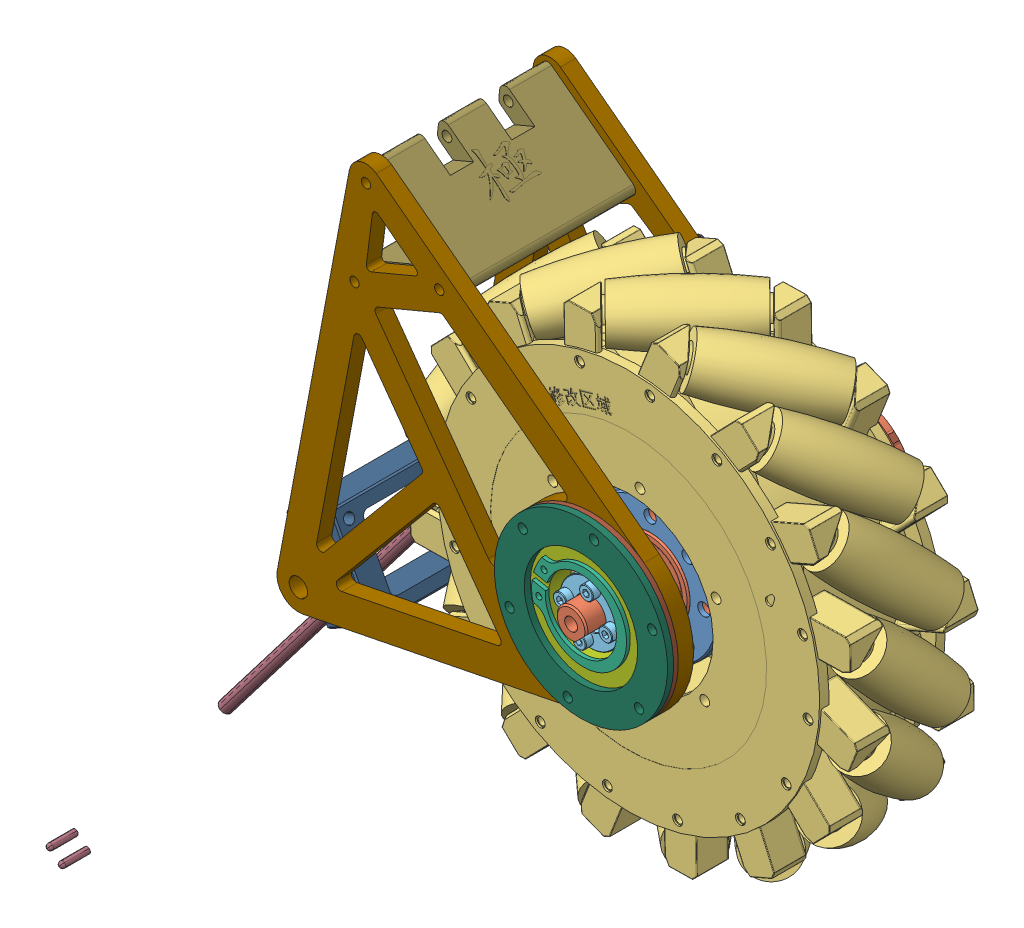
SolidWorks assembly 轮组1, configuration 默认. Lengths in mm.
Overall size (350.19 329.62 98.4).
20 component instances, 16 part files, 45 mates.
Components (placement in the parent):
- 轮组3508机加工件-1: 轮组3508机加工件 [默认] at origin size (56.5 56.5 41)
- RM3508直流无刷减速电机-1: RM3508直流无刷减速电机 [默认] at (-8.7166 16.154 -46.941) x (-0.922142 -0.386852 0) z (0 0 1) size (42 44.97 98.4)
- HEXROLL_16-D154-2.0-1: HEXROLL_16-D154-2.0 [默认] at (0 0 48.05) x (0.919361 0.393415 0) z (0 0 1) size (153.78 153.78 41)
- 轮组转动机加件-1: 轮组转动机加件 [默认] at (0 0 42.1) x (0 0 1) z (0.393415 -0.919361 0) size (22 67 67) (hidden)
- 轮组机加件-1: 轮组机加件 [默认] at (0 0 18) x (0 0 -1) z (0.8838 -0.467866 0) size (8 66 66)
- 胀紧套 ZZ21—10x20x13-1: 胀紧套 ZZ21—10x20x13 [默认] at (0 0 47.6) x (0.988286 -0.152615 0) z (0 0 1) size (20 20 15.5)
- GB894．2-86轴用弹性挡圈B型25-1: GB894．2-86轴用弹性挡圈B型25 [默认] at (0 0 62.2) x (-0.199141 -0.979971 0) z (0 0 1) size (28.2 30.93 1.2)
- 法兰轴承-1: 法兰轴承 [25*37*7-1.5] at (0 0 61.6) x (-0.301635 0.953423 0) z (-0.953423 -0.301635 0) size (40 7 40)
- 深沟球轴承-1: 深沟球轴承 [45x58x7] at (0 0 10) x (0.721643 -0.692266 0) z (-0.692266 -0.721643 0) size (58 7 58)
- 轮组转板-1: 轮组转板 [内侧板] at (-73.5991 84.4225 -2.5) x (-0.984808 0.173648 0) z (0 0 -1) size (120.47 137.51 5)
- 轮组转板-2: 轮组转板 [外侧板] at (-73.5991 84.4225 57.6) x (-0.984808 0.173648 0) z (0 0 -1) size (120.47 137.51 5)
- 轮组转点机加工件-1: 轮组转点机加工件 [默认] at (-95.6744 -40.7726 27.55) x (0 0 1) z (-0.888839 -0.45822 0) size (45 30 17)
- 轮组垫块-1: 轮组垫块 [默认] at (0 0 60.1) x (0.984808 -0.173648 0) z (0 0 1) size (56.5 56.5 1.5)
- 悬挂安装打印件-1: 悬挂安装打印件 [默认] at (-73.5991 84.4225 27.5) x (0.921941 0.38733 0) z (0 0 1) size (37.46 32.98 55)
- C620无刷电机调速器-2: C620无刷电机调速器 [默认] at (-74.3326 -5.2942 -10.4) x (0.607408 0.79439 0) z (0.79439 -0.607408 0) size (343.45 13.81 26.13)
- 深沟球轴承-2: 深沟球轴承 [6x13x5] at (-95.6744 -40.7726 5.05) x (-0.458973 -0.88845 0) z (-0.88845 0.458973 0) size (13 5 13)
- 深沟球轴承-3: 深沟球轴承 [6x13x5] at (-95.6744 -40.7726 45.05) x (0.999149 0.04124 0) z (0.04124 -0.999149 0) size (13 5 13)
- 推力球轴承-1: 推力球轴承 [F6-14M 6*14*5] at (-95.6744 -40.7726 0.05) x (0.246634 -0.969109 0) z (-0.969109 -0.246634 0) size (14 5 14)
- 推力球轴承-2: 推力球轴承 [F6-14M 6*14*5] at (-95.6744 -40.7726 50.05) x (0.140865 -0.990029 0) z (-0.990029 -0.140865 0) size (14 5 14)
- 轮组轴承压板-1: 轮组轴承压板 [默认] at (0 0 61.6) x (0.984808 -0.173648 0) z (0 0 1) size (56.5 56.5 2)
Mates (geometry in assembly coordinates):
- 同心1: concentric aligned: cylinder of 轮组3508机加工件-1 through (0 0 41) axis (0 0 -1) radius 21.05; cylinder of RM3508直流无刷减速电机-1 through (0 0 29.5) axis (0 0 -1) radius 21
- 重合1: coincident anti-aligned: plane of 轮组3508机加工件-1 through (0 0 39.5) normal (0 0 -1); plane of RM3508直流无刷减速电机-1 through (0 13 39.5) normal (0 0 1)
- 同心2: concentric anti-aligned: cylinder of 轮组3508机加工件-1 through (0 0 17) axis (0 0 -1) radius 22.5; cylinder of HEXROLL_16-D154-2.0-1 through (0 0 38) axis (0 0 1) radius 27.55
- 同心3: concentric anti-aligned: cylinder of RM3508直流无刷减速电机-1 through (0 0 66.8) axis (0 0 1) radius 5; cylinder of 轮组转动机加件-1 through (0 0 42.1) axis (0 0 -1) radius 13.5
- 重合2: coincident anti-aligned: plane of HEXROLL_16-D154-2.0-1 through (0 0 45.1) normal (0 0 -1); plane of 轮组转动机加件-1 through (-25.2824 -10.8189 45.1) normal (0 0 1)
- 同心4: concentric aligned: cylinder of HEXROLL_16-D154-2.0-1 through (-28.5002 -12.1959 40.5745) axis (0 0 1) radius 1.6; cylinder of 轮组转动机加件-1 through (-28.5002 -12.1959 45.1) axis (0 0 1) radius 1.25
- 同心5: concentric anti-aligned: cylinder of 轮组3508机加工件-1 through (0 0 41) axis (0 0 -1) radius 22.25; cylinder of 轮组机加件-1 through (0 0 18) axis (0 0 1) radius 33
- 重合3: coincident anti-aligned: plane of 轮组3508机加工件-1 through (0 0 10) normal (0 0 1); plane of 轮组机加件-1 through (15.4396 29.1654 10) normal (0 0 -1)
- 重合4: coincident anti-aligned: plane of HEXROLL_16-D154-2.0-1 through (0 0 10) normal (0 0 1); plane of 轮组机加件-1 through (15.4396 29.1654 10) normal (0 0 -1)
- 同心6: concentric anti-aligned: cylinder of RM3508直流无刷减速电机-1 through (0 0 66.8) axis (0 0 1) radius 5; cylinder of 胀紧套 ZZ21—10x20x13-1 through (0 0 60.6) axis (0 0 -1) radius 10
- 重合5: coincident anti-aligned: plane of 轮组转动机加件-1 through (-12.4114 -5.3111 62.8) normal (0 0 -1); plane of GB894．2-86轴用弹性挡圈B型25-1 through (-0.8134 0.1653 62.8) normal (0 0 1)
- 同心8: concentric aligned: cylinder of 轮组转动机加件-1 through (0 0 42.1) axis (0 0 -1) radius 11.6; cylinder of GB894．2-86轴用弹性挡圈B型25-1 through (0 0 62.8) axis (0 0 -1) radius 14.1
- 同心9: concentric aligned: cylinder of 轮组转动机加件-1 through (0 0 54.6) axis (0 0 1) radius 12.5; cylinder of 法兰轴承-1 through (0 0 54.6) axis (0 0 1) radius 18.5
- 重合6: coincident anti-aligned: plane of GB894．2-86轴用弹性挡圈B型25-1 through (-0.8134 0.1653 61.6) normal (0 0 -1); plane of 法兰轴承-1 through (0 0 61.6) normal (0 0 1)
- 重合7: coincident anti-aligned: plane of 轮组机加件-1 through (13.5681 25.6302 17) normal (0 0 -1); plane of 深沟球轴承-1 through (0 0 17) normal (0 0 1)
- 同心10: concentric anti-aligned: cylinder of 轮组机加件-1 through (0 0 18) axis (0 0 1) radius 33; cylinder of 深沟球轴承-1 through (0 0 17) axis (0 0 -1) radius 29
- 重合8: coincident anti-aligned: plane of 轮组3508机加工件-1 through (0 0 0) normal (0 0 -1); plane of 轮组转板-1 through (0 0 0) normal (0 0 1)
- 同心11: concentric anti-aligned: cylinder of 轮组3508机加工件-1 through (0 0 4) axis (0 0 -1) radius 28.25; cylinder of 轮组转板-1 through (0 0 -5) axis (0 0 1) radius 21.05
- 同心13: concentric anti-aligned: cylinder of 轮组3508机加工件-1 through (0 25.5 4) axis (0 0 1) radius 1.65; cylinder of 轮组转板-1 through (0 25.5 5) axis (0 0 -1) radius 1.525
- 同心15: concentric aligned: cylinder of 法兰轴承-1 through (0 0 54.6) axis (0 0 1) radius 18.5; cylinder of 轮组转板-2 through (0 0 55.1) axis (0 0 1) radius 18.5
- 重合9: coincident anti-aligned: plane of 法兰轴承-1 through (0 0 60.1) normal (0 0 -1); plane of 轮组转板-2 through (0 0 60.1) normal (0 0 1)
- 同心16: concentric aligned: cylinder of 轮组转板-1 through (-73.5991 84.4225 -5) axis (0 0 1) radius 1.525; cylinder of 轮组转板-2 through (-73.5991 84.4225 55.1) axis (0 0 1) radius 1.525
- 同心17: concentric aligned: cylinder of 轮组转板-1 through (-95.6744 -40.7726 -5) axis (0 0 1) radius 3; cylinder of 轮组转点机加工件-1 through (-95.6744 -40.7726 -7.95) axis (0 0 1) radius 4
- 宽度1: width anti-aligned: plane of 轮组转板-1 through (0 0 0) normal (0 0 1); plane of 轮组转点机加工件-1 through (0 0 55.1) normal (0 0 -1); plane of 轮组转板-2 through (-96.3563 -58 5.05) normal (0 0 -1); plane of 轮组转点机加工件-1 through (-96.3563 -58 50.05) normal (0 0 1)
- 重合10: coincident anti-aligned: plane of 轮组转板-2 through (0 0 60.1) normal (0 0 1); plane of 轮组垫块-1 through (0 0 60.1) normal (0 0 -1)
- 同心18: concentric anti-aligned: cylinder of 法兰轴承-1 through (0 0 60.1) axis (0 0 1) radius 20; cylinder of 轮组垫块-1 through (0 0 61.6) axis (0 0 -1) radius 28.25
- 同心19: concentric anti-aligned: cylinder of 轮组转板-1 through (-73.5991 84.4225 -5) axis (0 0 1) radius 1.525; cylinder of 悬挂安装打印件-1 through (-73.5991 84.4225 55) axis (0 0 -1) radius 1.6
- 同心20: concentric aligned: cylinder of 轮组转板-1 through (-77.3651 54.6599 26.54) axis (0 0 -1) radius 1.525; cylinder of 悬挂安装打印件-1 through (-77.3651 54.6599 55) axis (0 0 -1) radius 1.6
- 重合13: coincident anti-aligned: plane of 轮组转板-1 through (0 0 -5) normal (0 0 -1); plane of C620无刷电机调速器-2 through (-75.3652 -6.6447 -5) normal (0 0 1)
- 同心21: concentric aligned: cylinder of 轮组转点机加工件-1 through (-95.6744 -40.7726 10.05) axis (0 0 -1) radius 6.5; cylinder of 深沟球轴承-2 through (-95.6744 -40.7726 10.05) axis (0 0 -1) radius 6.5
- 重合14: coincident anti-aligned: plane of 轮组转点机加工件-1 through (-95.6744 -40.7726 10.05) normal (0 0 -1); plane of 深沟球轴承-2 through (-95.6744 -40.7726 10.05) normal (0 0 1)
- 同心22: concentric anti-aligned: cylinder of 轮组转点机加工件-1 through (-95.6744 -40.7726 45.05) axis (0 0 1) radius 6.5; cylinder of 深沟球轴承-3 through (-95.6744 -40.7726 50.05) axis (0 0 -1) radius 6.5
- 重合15: coincident anti-aligned: plane of 轮组转点机加工件-1 through (-95.6744 -40.7726 45.05) normal (0 0 1); plane of 深沟球轴承-3 through (-95.6744 -40.7726 45.05) normal (0 0 -1)
- 同心23: concentric anti-aligned: cylinder of 轮组转板-1 through (-95.6744 -40.7726 -5) axis (0 0 1) radius 3; cylinder of 推力球轴承-1 through (-95.6744 -40.7726 5.05) axis (0 0 -1) radius 3
- 重合16: coincident anti-aligned: plane of 轮组转点机加工件-1 through (-96.3563 -58 5.05) normal (0 0 -1); plane of 推力球轴承-1 through (-95.6744 -40.7726 5.05) normal (0 0 1)
- 同心24: concentric anti-aligned: cylinder of 轮组转点机加工件-1 through (-95.6744 -40.7726 -7.95) axis (0 0 1) radius 4; cylinder of 推力球轴承-2 through (-95.6744 -40.7726 55.05) axis (0 0 -1) radius 7
- 重合17: coincident anti-aligned: plane of 轮组转点机加工件-1 through (-96.3563 -58 50.05) normal (0 0 1); plane of 推力球轴承-2 through (-95.6744 -40.7726 50.05) normal (0 0 -1)
- 平行1: parallel aligned: plane of 轮组转板-1 through (-55.2581 4.2183 -66.4021) normal (0.79439 -0.607408 0); plane of C620无刷电机调速器-2 through (-77.5694 -30.7652 -6) normal (0.79439 -0.607408 0)
- 同心25: concentric anti-aligned: cylinder of 轮组转板-2 through (4.2978 24.374 65.1) axis (0 0 -1) radius 1.525; cylinder of 轮组垫块-1 through (4.2978 24.374 55.5745) axis (0 0 1) radius 1.6
- 同心26: concentric aligned: cylinder of 轮组垫块-1 through (0 0 61.6) axis (0 0 -1) radius 28.25; cylinder of 轮组轴承压板-1 through (0 0 63.6) axis (0 0 -1) radius 28.25
- 重合18: coincident anti-aligned: plane of 轮组垫块-1 through (0 0 61.6) normal (0 0 1); plane of 轮组轴承压板-1 through (0 0 61.6) normal (0 0 -1)
- 同心27: concentric anti-aligned: cylinder of 轮组转板-2 through (-23.2574 -8.465 65.1) axis (0 0 -1) radius 1.525; cylinder of 轮组轴承压板-1 through (-23.2574 -8.465 61.6) axis (0 0 1) radius 1.525
- 重合19: coincident anti-aligned: plane of 轮组转板-1 through (0 0 0) normal (0 0 1); plane of 悬挂安装打印件-1 through (-73.5991 84.4225 0) normal (0 0 -1)
- 距离1: distance = 3.5 mm aligned: plane of 胀紧套 ZZ21—10x20x13-1 through (0 0 60.6) normal (0 0 1); plane of 轮组转动机加件-1 through (-9.1936 -3.9341 64.1) normal (0 0 1)
- 同心28: concentric anti-aligned: cylinder of 轮组3508机加工件-1 through (12.3744 12.3744 46.5) axis (0 0 -1) radius 2; cylinder of RM3508直流无刷减速电机-1 through (12.3744 12.3744 39.5) axis (0 0 1) radius 1.65
